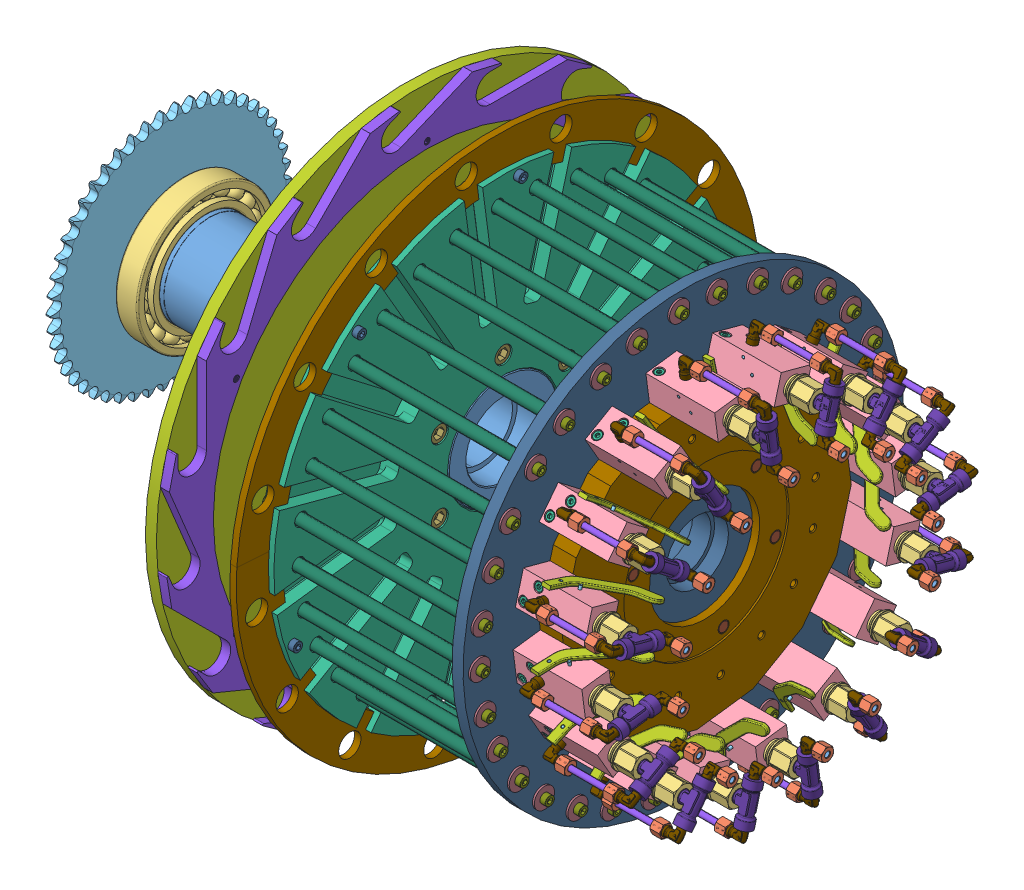
SolidWorks assembly assieme parte rotante, configuration Default. Lengths in mm.
Overall size (749.63 778.63 778.63).
555 component instances, 28 part files, 76 mates.
Components (placement in the parent):
- albero rotazione piatti-1: albero rotazione piatti [Default] at (60.413 18.3637 415) size (415 200 200)
- seger 100mm-2: seger 100mm [KS 1336 E - 100] at (-146.4567 18.3637 415) x (0 0 -1) z (1 0 0) size (107.55 112.98 3)
- SKF - 6020 - 20,DE,NC,20_68-1: SKF - 6020 - 20,DE,NC,20_68 [SKF - 6020 - 20,DE,NC,20_68] at (-131.4567 18.3637 415) x (1 0 0) z (0 -0.434476 -0.900684) size (24 150 150)
- calettatore d95-1: calettatore d95 [Default] at (-173.8867 18.3637 415) size (39.5 135 135)
- Chain wheel ISO - 50Z 10A-1-1: Chain wheel ISO - 50Z 10A-1 [Chain wheel ISO - 50Z 10A-1 --50SB120H25L95.0N] at (-164.8867 18.3637 415) size (28.93 262.06 262.51)
- Disco supporto montaggio e Colonne-1: Disco supporto montaggio e Colonne [Default] at (204.0433 18.3637 415) x (0 -0.866025 -0.5) z (1 0 0) size (499.6 499.6 29)
- SKF - 6020 - 20,DE,NC,20_68-2: SKF - 6020 - 20,DE,NC,20_68 [SKF - 6020 - 20,DE,NC,20_68] at (62.0433 18.3637 415) x (1 0 0) z (0 -0.432628 -0.901573) size (24 150 150)
- piatto rotante porta tappi-1: piatto rotante porta tappi [Default] at (99.0433 18.3637 415) x (0 0 -1) z (1 0 0) size (570 570 20.57)
- disco trasportatore tappi 31-1: disco trasportatore tappi 31 [Default] at (111.0433 18.3637 415) x (0 0.5 -0.866025) z (1 0 0) size (570 570 10.42)
- Distributore Rotante-1: Distributore Rotante [Default] at (425.0433 18.3637 415) x (0 -0.258819 -0.965926) z (1 0 0) size (310 310 25.54)
- disco trascinato porta distributore vuoto-1: disco trascinato porta distributore vuoto [Default] at (400.0433 18.3637 415) x (0 0.258819 0.965926) z (-1 0 0) size (480 480 50)
- m12 35mm-1: m12 35mm [ISO 4762 M12 x 35 - 35N] at (376.0433 -58.9104 394.2945) x (1 0 0) z (0 -0.5 0.866025) size (47 18 18)
- m12 90mm-3: m12 90mm [ISO 4762 M12 x 90 - 90N] at (203.0433 -21.6363 345.718) x (-1 0 0) z (0 -0.5 0.866025) size (102 18 18)
- rondella M6-90: rondella M6 [Washer ISO 7094 - 6] at (99.0433 -101.6363 207.1539) x (1 0 0) z (0 -1 0) size (2 22 22)
- M6 20mm-1: M6 20mm [ISO 4762 M6 x 20 - 20N] at (91.0433 -101.6363 207.1539) x (1 0 0) z (0 0.5 0.866025) size (26 10 10)
- m12 35mm-2: m12 35mm [ISO 4762 M12 x 35 - 35N] at (376.0433 -2.3418 337.7259) x (1 0 0) z (0 -1 0) size (47 18 18)
- m12 35mm-3: m12 35mm [ISO 4762 M12 x 35 - 35N] at (376.0433 74.9322 358.4315) x (1 0 0) z (0 -0.5 -0.866025) size (47 18 18)
- m12 35mm-4: m12 35mm [ISO 4762 M12 x 35 - 35N] at (376.0433 95.6378 435.7055) x (1 0 0) z (0 0.5 -0.866025) size (47 18 18)
- m12 35mm-5: m12 35mm [ISO 4762 M12 x 35 - 35N] at (376.0433 39.0692 492.2741) x (1 0 0) z (0 1 0) size (47 18 18)
- m12 35mm-6: m12 35mm [ISO 4762 M12 x 35 - 35N] at (376.0433 -38.2048 471.5685) x (1 0 0) z (0 0.5 0.866025) size (47 18 18)
- rondella M6-91: rondella M6 [Washer ISO 7094 - 6] at (99.0433 138.3637 207.1539) x (1 0 0) z (0 -0.5 -0.866025) size (2 22 22)
- rondella M6-92: rondella M6 [Washer ISO 7094 - 6] at (99.0433 258.3637 415) x (1 0 0) z (0 0.5 -0.866025) size (2 22 22)
- rondella M6-93: rondella M6 [Washer ISO 7094 - 6] at (99.0433 138.3637 622.8461) x (1 0 0) z (0 1 0) size (2 22 22)
- rondella M6-94: rondella M6 [Washer ISO 7094 - 6] at (99.0433 -101.6363 622.8461) x (1 0 0) z (0 0.5 0.866025) size (2 22 22)
- rondella M6-95: rondella M6 [Washer ISO 7094 - 6] at (99.0433 -221.6363 415) x (1 0 0) z (0 -0.5 0.866025) size (2 22 22)
- M6 20mm-2: M6 20mm [ISO 4762 M6 x 20 - 20N] at (91.0433 138.3637 207.1539) x (1 0 0) z (0 -0.5 0.866025) size (26 10 10)
- M6 20mm-3: M6 20mm [ISO 4762 M6 x 20 - 20N] at (91.0433 258.3637 415) x (1 0 0) z (0 -1 0) size (26 10 10)
- M6 20mm-4: M6 20mm [ISO 4762 M6 x 20 - 20N] at (91.0433 138.3637 622.8461) x (1 0 0) z (0 -0.5 -0.866025) size (26 10 10)
- M6 20mm-5: M6 20mm [ISO 4762 M6 x 20 - 20N] at (91.0433 -101.6363 622.8461) x (1 0 0) z (0 0.5 -0.866025) size (26 10 10)
- M6 20mm-6: M6 20mm [ISO 4762 M6 x 20 - 20N] at (91.0433 -221.6363 415) x (1 0 0) z (0 1 0) size (26 10 10)
- m12 90mm-4: m12 90mm [ISO 4762 M12 x 90 - 90N] at (203.0433 58.3637 345.718) x (-1 0 0) z (0 -1 0) size (102 18 18)
- m12 90mm-5: m12 90mm [ISO 4762 M12 x 90 - 90N] at (203.0433 98.3637 415) x (-1 0 0) z (0 -0.5 -0.866025) size (102 18 18)
- m12 90mm-6: m12 90mm [ISO 4762 M12 x 90 - 90N] at (203.0433 58.3637 484.282) x (-1 0 0) z (0 0.5 -0.866025) size (102 18 18)
- m12 90mm-7: m12 90mm [ISO 4762 M12 x 90 - 90N] at (203.0433 -21.6363 484.282) x (-1 0 0) z (0 1 0) size (102 18 18)
- m12 90mm-8: m12 90mm [ISO 4762 M12 x 90 - 90N] at (203.0433 -61.6363 415) x (-1 0 0) z (0 0.5 0.866025) size (102 18 18)
- asta scorrimento carello-1: asta scorrimento carello [Default] at (287.5433 70.1437 197.9013) x (0 0 -1) z (1 0 0) size (12 12 225)
- rondella M6-74: rondella M6 [Washer ISO 7094 - 6] at (175.0433 70.1437 197.9013) x (1 0 0) z (0 -1 0) size (2 22 22)
- M6 16mm-1: M6 16mm [ISO 4762 M6 x 16 - 16N] at (167.0433 70.1437 197.9013) size (22 10 10)
- M6 16mm-2: M6 16mm [ISO 4762 M6 x 16 - 16N] at (408.0433 70.1437 197.9013) x (-1 0 0) z (0 0 -1) size (22 10 10)
- rondella M6-96: rondella M6 [Washer ISO 7094 - 6] at (400.0433 70.1437 197.9013) x (-1 0 0) z (0 1 0) size (2 22 22)
- rondella M6-112: rondella M6 [Washer ISO 7094 - 6] at (175.0433 24.5373 191.8971) x (1 0 0) z (0 -0.965926 -0.258819) size (2 22 22)
- M6 16mm-3: M6 16mm [ISO 4762 M6 x 16 - 16N] at (167.0433 24.5373 191.8971) x (1 0 0) z (0 0.258819 -0.965926) size (22 10 10)
- asta scorrimento carello-2: asta scorrimento carello [Default] at (287.5433 24.5373 191.8971) x (0 0.258819 -0.965926) z (-1 0 0) size (12 12 225)
- rondella M6-128: rondella M6 [Washer ISO 7094 - 6] at (400.0433 24.5373 191.8971) x (-1 0 0) z (0 0.965926 0.258819) size (2 22 22)
- M6 16mm-4: M6 16mm [ISO 4762 M6 x 16 - 16N] at (408.0433 24.5373 191.8971) x (-1 0 0) z (0 -0.258819 0.965926) size (22 10 10)
- AssiemeValvola-1: AssiemeValvola [Default] at (515.3257 40.5532 246.4544) x (0 -0.130526 0.991445) z (0 0.991445 0.130526) size (90.26 138.63 38)
  - RaccordoT-1: RaccordoT [Default] at origin size (43 29.75 16.5)
  - Raccordo a L-1: Raccordo a L [Default] at (-30 0 0) x (0 -1 0) z (0 0 -1) size (28.34 25.51 14.01)
    - 1809_06_10_01-1: 1809_06_10_01 [Default] at origin size (22.49 23 10)
    - 1809_06_10_02-1: 1809_06_10_02 [Default] at origin size (6.5 8.5 8.5)
    - 1809_06_10_03-1: 1809_06_10_03 [Default] at origin size (11.02 15.01 14.01)
  - Raccordo a L-2: Raccordo a L [Default] at (30 0 0) x (0 1 0) z (0 0 -1) size (28.34 25.51 14.01)
    - 1809_06_10_01-1: 1809_06_10_01 [Default] at origin size (22.49 23 10)
    - 1809_06_10_02-1: 1809_06_10_02 [Default] at origin size (6.5 8.5 8.5)
    - 1809_06_10_03-1: 1809_06_10_03 [Default] at origin size (11.02 15.01 14.01)
  - TappoChiusura-1: TappoChiusura [Default] at (0 -32 0) x (0 -1 0) z (0 0 1) size (38.28 26.74 26.74)
  - CorpoValvola-1: CorpoValvola [Default] at (-15 -115.2824 0) size (30 75 34)
  - Raccordo a L-3: Raccordo a L [Default] at (-30 -88.2824 0) x (0 1 0) z (0 0 1) size (28.34 25.51 14.01)
    - 1809_06_10_01-1: 1809_06_10_01 [Default] at origin size (22.49 23 10)
    - 1809_06_10_02-1: 1809_06_10_02 [Default] at origin size (6.5 8.5 8.5)
    - 1809_06_10_03-1: 1809_06_10_03 [Default] at origin size (11.02 15.01 14.01)
  - Spina_3x38-1: Spina_3x38 [Default] at (0 -68.2824 -21) x (-1 0 0) z (0 0 1) size (3 3 38)
  - Spina_3x38-2: Spina_3x38 [Default] at (-10 -80.2824 -21) x (0.996193 0.087174 0) z (0 0 1) size (3 3 38)
  - M5 40mm-3: M5 40mm [ISO 4762 M5 x 40 - 40N] at (-14.6 -108.7824 9) size (45 8.5 8.5)
  - M5 40mm-2: M5 40mm [ISO 4762 M5 x 40 - 40N] at (-14.6 -96.7824 -9) size (45 8.5 8.5)
  - LevaValvola-1: LevaValvola [Default] at (-24.507 -86.571 -17) x (0.996193 0.087174 0) z (0 0 1) size (77.55 60.2 4)
  - Tubo-1: Tubo [Default] at (-30 -15.9665 0) x (1 0 0) z (0 -1 0) size (6 6 56.4)
- M6 16mm-5: M6 16mm [ISO 4762 M6 x 16 - 16N] at (167.0433 -16.8778 194.6116) x (1 0 0) z (0 0.382683 0.92388) size (22 10 10)
- M6 16mm-6: M6 16mm [ISO 4762 M6 x 16 - 16N] at (167.0433 -98.5342 224.874) x (1 0 0) z (0 0.707107 0.707107) size (22 10 10)
- M6 16mm-7: M6 16mm [ISO 4762 M6 x 16 - 16N] at (167.0433 -162.3939 284.0814) x (1 0 0) z (0 0.92388 0.382683) size (22 10 10)
- M6 16mm-8: M6 16mm [ISO 4762 M6 x 16 - 16N] at (167.0433 -198.735 363.22) x (1 0 0) z (0 1 0) size (22 10 10)
- M6 16mm-9: M6 16mm [ISO 4762 M6 x 16 - 16N] at (167.0433 -202.0247 450.2415) x (1 0 0) z (0 0.92388 -0.382683) size (22 10 10)
- M6 16mm-10: M6 16mm [ISO 4762 M6 x 16 - 16N] at (167.0433 -171.7623 531.8979) x (1 0 0) z (0 0.707107 -0.707107) size (22 10 10)
- M6 16mm-11: M6 16mm [ISO 4762 M6 x 16 - 16N] at (167.0433 -112.5549 595.7576) x (1 0 0) z (0 0.382683 -0.92388) size (22 10 10)
- M6 16mm-12: M6 16mm [ISO 4762 M6 x 16 - 16N] at (167.0433 -33.4163 632.0987) x (1 0 0) z (0 0 -1) size (22 10 10)
- M6 16mm-13: M6 16mm [ISO 4762 M6 x 16 - 16N] at (167.0433 53.6052 635.3884) x (1 0 0) z (0 -0.382683 -0.92388) size (22 10 10)
- M6 16mm-14: M6 16mm [ISO 4762 M6 x 16 - 16N] at (167.0433 135.2616 605.126) x (1 0 0) z (0 -0.707107 -0.707107) size (22 10 10)
- M6 16mm-15: M6 16mm [ISO 4762 M6 x 16 - 16N] at (167.0433 199.1213 545.9186) x (1 0 0) z (0 -0.92388 -0.382683) size (22 10 10)
- M6 16mm-16: M6 16mm [ISO 4762 M6 x 16 - 16N] at (167.0433 235.4624 466.78) x (1 0 0) z (0 -1 0) size (22 10 10)
- M6 16mm-17: M6 16mm [ISO 4762 M6 x 16 - 16N] at (167.0433 238.7521 379.7585) x (1 0 0) z (0 -0.92388 0.382683) size (22 10 10)
- M6 16mm-18: M6 16mm [ISO 4762 M6 x 16 - 16N] at (167.0433 208.4897 298.1021) x (1 0 0) z (0 -0.707107 0.707107) size (22 10 10)
- M6 16mm-19: M6 16mm [ISO 4762 M6 x 16 - 16N] at (167.0433 149.2823 234.2424) x (1 0 0) z (0 -0.382683 0.92388) size (22 10 10)
- rondella M6-75: rondella M6 [Washer ISO 7094 - 6] at (175.0433 -16.8778 194.6116) x (1 0 0) z (0 -0.92388 0.382683) size (2 22 22)
- rondella M6-76: rondella M6 [Washer ISO 7094 - 6] at (175.0433 -98.5342 224.874) x (1 0 0) z (0 -0.707107 0.707107) size (2 22 22)
- rondella M6-77: rondella M6 [Washer ISO 7094 - 6] at (175.0433 -162.3939 284.0814) x (1 0 0) z (0 -0.382683 0.92388) size (2 22 22)
- rondella M6-78: rondella M6 [Washer ISO 7094 - 6] at (175.0433 -198.735 363.22) size (2 22 22)
- rondella M6-79: rondella M6 [Washer ISO 7094 - 6] at (175.0433 -202.0247 450.2415) x (1 0 0) z (0 0.382683 0.92388) size (2 22 22)
- rondella M6-80: rondella M6 [Washer ISO 7094 - 6] at (175.0433 -171.7623 531.8979) x (1 0 0) z (0 0.707107 0.707107) size (2 22 22)
- rondella M6-81: rondella M6 [Washer ISO 7094 - 6] at (175.0433 -112.5549 595.7576) x (1 0 0) z (0 0.92388 0.382683) size (2 22 22)
- rondella M6-82: rondella M6 [Washer ISO 7094 - 6] at (175.0433 -33.4163 632.0987) x (1 0 0) z (0 1 0) size (2 22 22)
- rondella M6-83: rondella M6 [Washer ISO 7094 - 6] at (175.0433 53.6052 635.3884) x (1 0 0) z (0 0.92388 -0.382683) size (2 22 22)
- rondella M6-84: rondella M6 [Washer ISO 7094 - 6] at (175.0433 135.2616 605.126) x (1 0 0) z (0 0.707107 -0.707107) size (2 22 22)
- rondella M6-85: rondella M6 [Washer ISO 7094 - 6] at (175.0433 199.1213 545.9186) x (1 0 0) z (0 0.382683 -0.92388) size (2 22 22)
- rondella M6-86: rondella M6 [Washer ISO 7094 - 6] at (175.0433 235.4624 466.78) x (1 0 0) z (0 0 -1) size (2 22 22)
- rondella M6-87: rondella M6 [Washer ISO 7094 - 6] at (175.0433 238.7521 379.7585) x (1 0 0) z (0 -0.382683 -0.92388) size (2 22 22)
- rondella M6-88: rondella M6 [Washer ISO 7094 - 6] at (175.0433 208.4897 298.1021) x (1 0 0) z (0 -0.707107 -0.707107) size (2 22 22)
- rondella M6-89: rondella M6 [Washer ISO 7094 - 6] at (175.0433 149.2823 234.2424) x (1 0 0) z (0 -0.92388 -0.382683) size (2 22 22)
- asta scorrimento carello-3: asta scorrimento carello [Default] at (287.5433 -16.8778 194.6116) x (0 -0.382683 -0.92388) z (1 0 0) size (12 12 225)
- asta scorrimento carello-4: asta scorrimento carello [Default] at (287.5433 -98.5342 224.874) x (0 -0.707107 -0.707107) z (1 0 0) size (12 12 225)
- asta scorrimento carello-5: asta scorrimento carello [Default] at (287.5433 -162.3939 284.0814) x (0 -0.92388 -0.382683) z (1 0 0) size (12 12 225)
- asta scorrimento carello-6: asta scorrimento carello [Default] at (287.5433 -198.735 363.22) x (0 -1 0) z (1 0 0) size (12 12 225)
- asta scorrimento carello-7: asta scorrimento carello [Default] at (287.5433 -202.0247 450.2415) x (0 -0.92388 0.382683) z (1 0 0) size (12 12 225)
- asta scorrimento carello-8: asta scorrimento carello [Default] at (287.5433 -171.7623 531.8979) x (0 -0.707107 0.707107) z (1 0 0) size (12 12 225)
- asta scorrimento carello-9: asta scorrimento carello [Default] at (287.5433 -112.5549 595.7576) x (0 -0.382683 0.92388) z (1 0 0) size (12 12 225)
- asta scorrimento carello-10: asta scorrimento carello [Default] at (287.5433 -33.4163 632.0987) x (0 0 1) z (1 0 0) size (12 12 225)
- asta scorrimento carello-11: asta scorrimento carello [Default] at (287.5433 53.6052 635.3884) x (0 0.382683 0.92388) z (1 0 0) size (12 12 225)
- asta scorrimento carello-12: asta scorrimento carello [Default] at (287.5433 135.2616 605.126) x (0 0.707107 0.707107) z (1 0 0) size (12 12 225)
- asta scorrimento carello-13: asta scorrimento carello [Default] at (287.5433 199.1213 545.9186) x (0 0.92388 0.382683) z (1 0 0) size (12 12 225)
- asta scorrimento carello-14: asta scorrimento carello [Default] at (287.5433 235.4624 466.78) x (0 1 0) z (1 0 0) size (12 12 225)
- asta scorrimento carello-15: asta scorrimento carello [Default] at (287.5433 238.7521 379.7585) x (0 0.92388 -0.382683) z (1 0 0) size (12 12 225)
- asta scorrimento carello-16: asta scorrimento carello [Default] at (287.5433 208.4897 298.1021) x (0 0.707107 -0.707107) z (1 0 0) size (12 12 225)
- asta scorrimento carello-17: asta scorrimento carello [Default] at (287.5433 149.2823 234.2424) x (0 0.382683 -0.92388) z (1 0 0) size (12 12 225)
- M6 16mm-20: M6 16mm [ISO 4762 M6 x 16 - 16N] at (408.0433 -16.8778 194.6116) x (-1 0 0) z (0 -0.382683 -0.92388) size (22 10 10)
- M6 16mm-21: M6 16mm [ISO 4762 M6 x 16 - 16N] at (408.0433 -98.5342 224.874) x (-1 0 0) z (0 -0.707107 -0.707107) size (22 10 10)
- M6 16mm-22: M6 16mm [ISO 4762 M6 x 16 - 16N] at (408.0433 -162.3939 284.0814) x (-1 0 0) z (0 -0.92388 -0.382683) size (22 10 10)
- M6 16mm-23: M6 16mm [ISO 4762 M6 x 16 - 16N] at (408.0433 -198.735 363.22) x (-1 0 0) z (0 -1 0) size (22 10 10)
- M6 16mm-24: M6 16mm [ISO 4762 M6 x 16 - 16N] at (408.0433 -202.0247 450.2415) x (-1 0 0) z (0 -0.92388 0.382683) size (22 10 10)
- M6 16mm-25: M6 16mm [ISO 4762 M6 x 16 - 16N] at (408.0433 -171.7623 531.8979) x (-1 0 0) z (0 -0.707107 0.707107) size (22 10 10)
- M6 16mm-26: M6 16mm [ISO 4762 M6 x 16 - 16N] at (408.0433 -112.5549 595.7576) x (-1 0 0) z (0 -0.382683 0.92388) size (22 10 10)
- M6 16mm-27: M6 16mm [ISO 4762 M6 x 16 - 16N] at (408.0433 -33.4163 632.0987) x (-1 0 0) z (0 0 1) size (22 10 10)
- M6 16mm-28: M6 16mm [ISO 4762 M6 x 16 - 16N] at (408.0433 53.6052 635.3884) x (-1 0 0) z (0 0.382683 0.92388) size (22 10 10)
- M6 16mm-29: M6 16mm [ISO 4762 M6 x 16 - 16N] at (408.0433 135.2616 605.126) x (-1 0 0) z (0 0.707107 0.707107) size (22 10 10)
- M6 16mm-30: M6 16mm [ISO 4762 M6 x 16 - 16N] at (408.0433 199.1213 545.9186) x (-1 0 0) z (0 0.92388 0.382683) size (22 10 10)
- M6 16mm-31: M6 16mm [ISO 4762 M6 x 16 - 16N] at (408.0433 235.4624 466.78) x (-1 0 0) z (0 1 0) size (22 10 10)
- M6 16mm-32: M6 16mm [ISO 4762 M6 x 16 - 16N] at (408.0433 238.7521 379.7585) x (-1 0 0) z (0 0.92388 -0.382683) size (22 10 10)
- M6 16mm-33: M6 16mm [ISO 4762 M6 x 16 - 16N] at (408.0433 208.4897 298.1021) x (-1 0 0) z (0 0.707107 -0.707107) size (22 10 10)
- M6 16mm-34: M6 16mm [ISO 4762 M6 x 16 - 16N] at (408.0433 149.2823 234.2424) x (-1 0 0) z (0 0.382683 -0.92388) size (22 10 10)
- rondella M6-97: rondella M6 [Washer ISO 7094 - 6] at (400.0433 -16.8778 194.6116) x (-1 0 0) z (0 0.92388 -0.382683) size (2 22 22)
- rondella M6-98: rondella M6 [Washer ISO 7094 - 6] at (400.0433 -98.5342 224.874) x (-1 0 0) z (0 0.707107 -0.707107) size (2 22 22)
- rondella M6-99: rondella M6 [Washer ISO 7094 - 6] at (400.0433 -162.3939 284.0814) x (-1 0 0) z (0 0.382683 -0.92388) size (2 22 22)
- rondella M6-100: rondella M6 [Washer ISO 7094 - 6] at (400.0433 -198.735 363.22) x (-1 0 0) z (0 0 -1) size (2 22 22)
- rondella M6-101: rondella M6 [Washer ISO 7094 - 6] at (400.0433 -202.0247 450.2415) x (-1 0 0) z (0 -0.382683 -0.92388) size (2 22 22)
- rondella M6-102: rondella M6 [Washer ISO 7094 - 6] at (400.0433 -171.7623 531.8979) x (-1 0 0) z (0 -0.707107 -0.707107) size (2 22 22)
- rondella M6-103: rondella M6 [Washer ISO 7094 - 6] at (400.0433 -112.5549 595.7576) x (-1 0 0) z (0 -0.92388 -0.382683) size (2 22 22)
- rondella M6-104: rondella M6 [Washer ISO 7094 - 6] at (400.0433 -33.4163 632.0987) x (-1 0 0) z (0 -1 0) size (2 22 22)
- rondella M6-105: rondella M6 [Washer ISO 7094 - 6] at (400.0433 53.6052 635.3884) x (-1 0 0) z (0 -0.92388 0.382683) size (2 22 22)
- rondella M6-106: rondella M6 [Washer ISO 7094 - 6] at (400.0433 135.2616 605.126) x (-1 0 0) z (0 -0.707107 0.707107) size (2 22 22)
- rondella M6-107: rondella M6 [Washer ISO 7094 - 6] at (400.0433 199.1213 545.9186) x (-1 0 0) z (0 -0.382683 0.92388) size (2 22 22)
- rondella M6-108: rondella M6 [Washer ISO 7094 - 6] at (400.0433 235.4624 466.78) x (-1 0 0) z (0 0 1) size (2 22 22)
- rondella M6-109: rondella M6 [Washer ISO 7094 - 6] at (400.0433 238.7521 379.7585) x (-1 0 0) z (0 0.382683 0.92388) size (2 22 22)
- rondella M6-110: rondella M6 [Washer ISO 7094 - 6] at (400.0433 208.4897 298.1021) x (-1 0 0) z (0 0.707107 0.707107) size (2 22 22)
- rondella M6-111: rondella M6 [Washer ISO 7094 - 6] at (400.0433 149.2823 234.2424) x (-1 0 0) z (0 0.92388 0.382683) size (2 22 22)
- rondella M6-113: rondella M6 [Washer ISO 7094 - 6] at (175.0433 -61.3104 206.5173) x (1 0 0) z (0 -0.991445 0.130526) size (2 22 22)
- rondella M6-114: rondella M6 [Washer ISO 7094 - 6] at (175.0433 -135.0285 252.8771) x (1 0 0) z (0 -0.866025 0.5) size (2 22 22)
- rondella M6-115: rondella M6 [Washer ISO 7094 - 6] at (175.0433 -185.3939 323.9186) x (1 0 0) z (0 -0.608761 0.793353) size (2 22 22)
- rondella M6-116: rondella M6 [Washer ISO 7094 - 6] at (175.0433 -204.7392 408.8264) x (1 0 0) z (0 -0.258819 0.965926) size (2 22 22)
- rondella M6-117: rondella M6 [Washer ISO 7094 - 6] at (175.0433 -190.119 494.6741) x (1 0 0) z (0 0.130526 0.991445) size (2 22 22)
- rondella M6-118: rondella M6 [Washer ISO 7094 - 6] at (175.0433 -143.7592 568.3922) x (1 0 0) z (0 0.5 0.866025) size (2 22 22)
- rondella M6-119: rondella M6 [Washer ISO 7094 - 6] at (175.0433 -72.7177 618.7576) x (1 0 0) z (0 0.793353 0.608761) size (2 22 22)
- rondella M6-120: rondella M6 [Washer ISO 7094 - 6] at (175.0433 12.1901 638.1029) x (1 0 0) z (0 0.965926 0.258819) size (2 22 22)
- rondella M6-121: rondella M6 [Washer ISO 7094 - 6] at (175.0433 98.0378 623.4827) x (1 0 0) z (0 0.991445 -0.130526) size (2 22 22)
- rondella M6-122: rondella M6 [Washer ISO 7094 - 6] at (175.0433 171.7559 577.1229) x (1 0 0) z (0 0.866025 -0.5) size (2 22 22)
- rondella M6-123: rondella M6 [Washer ISO 7094 - 6] at (175.0433 222.1213 506.0814) x (1 0 0) z (0 0.608761 -0.793353) size (2 22 22)
- rondella M6-124: rondella M6 [Washer ISO 7094 - 6] at (175.0433 241.4666 421.1736) x (1 0 0) z (0 0.258819 -0.965926) size (2 22 22)
- rondella M6-125: rondella M6 [Washer ISO 7094 - 6] at (175.0433 226.8464 335.3259) x (1 0 0) z (0 -0.130526 -0.991445) size (2 22 22)
- rondella M6-126: rondella M6 [Washer ISO 7094 - 6] at (175.0433 180.4866 261.6078) x (1 0 0) z (0 -0.5 -0.866025) size (2 22 22)
- rondella M6-127: rondella M6 [Washer ISO 7094 - 6] at (175.0433 109.4451 211.2424) x (1 0 0) z (0 -0.793353 -0.608761) size (2 22 22)
- M6 16mm-35: M6 16mm [ISO 4762 M6 x 16 - 16N] at (167.0433 -61.3104 206.5173) x (1 0 0) z (0 -0.130526 -0.991445) size (22 10 10)
- M6 16mm-36: M6 16mm [ISO 4762 M6 x 16 - 16N] at (167.0433 -135.0285 252.8771) x (1 0 0) z (0 -0.5 -0.866025) size (22 10 10)
- M6 16mm-37: M6 16mm [ISO 4762 M6 x 16 - 16N] at (167.0433 -185.3939 323.9186) x (1 0 0) z (0 -0.793353 -0.608761) size (22 10 10)
- M6 16mm-38: M6 16mm [ISO 4762 M6 x 16 - 16N] at (167.0433 -204.7392 408.8264) x (1 0 0) z (0 -0.965926 -0.258819) size (22 10 10)
- M6 16mm-39: M6 16mm [ISO 4762 M6 x 16 - 16N] at (167.0433 -190.119 494.6741) x (1 0 0) z (0 -0.991445 0.130526) size (22 10 10)
- M6 16mm-40: M6 16mm [ISO 4762 M6 x 16 - 16N] at (167.0433 -143.7592 568.3922) x (1 0 0) z (0 -0.866025 0.5) size (22 10 10)
- M6 16mm-41: M6 16mm [ISO 4762 M6 x 16 - 16N] at (167.0433 -72.7177 618.7576) x (1 0 0) z (0 -0.608761 0.793353) size (22 10 10)
- M6 16mm-42: M6 16mm [ISO 4762 M6 x 16 - 16N] at (167.0433 12.1901 638.1029) x (1 0 0) z (0 -0.258819 0.965926) size (22 10 10)
- M6 16mm-43: M6 16mm [ISO 4762 M6 x 16 - 16N] at (167.0433 98.0378 623.4827) x (1 0 0) z (0 0.130526 0.991445) size (22 10 10)
- M6 16mm-44: M6 16mm [ISO 4762 M6 x 16 - 16N] at (167.0433 171.7559 577.1229) x (1 0 0) z (0 0.5 0.866025) size (22 10 10)
- M6 16mm-45: M6 16mm [ISO 4762 M6 x 16 - 16N] at (167.0433 222.1213 506.0814) x (1 0 0) z (0 0.793353 0.608761) size (22 10 10)
- M6 16mm-46: M6 16mm [ISO 4762 M6 x 16 - 16N] at (167.0433 241.4666 421.1736) x (1 0 0) z (0 0.965926 0.258819) size (22 10 10)
- M6 16mm-47: M6 16mm [ISO 4762 M6 x 16 - 16N] at (167.0433 226.8464 335.3259) x (1 0 0) z (0 0.991445 -0.130526) size (22 10 10)
- M6 16mm-48: M6 16mm [ISO 4762 M6 x 16 - 16N] at (167.0433 180.4866 261.6078) x (1 0 0) z (0 0.866025 -0.5) size (22 10 10)
- M6 16mm-49: M6 16mm [ISO 4762 M6 x 16 - 16N] at (167.0433 109.4451 211.2424) x (1 0 0) z (0 0.608761 -0.793353) size (22 10 10)
- asta scorrimento carello-18: asta scorrimento carello [Default] at (287.5433 -61.3104 206.5173) x (0 -0.130526 -0.991445) z (-1 0 0) size (12 12 225)
- asta scorrimento carello-19: asta scorrimento carello [Default] at (287.5433 -135.0285 252.8771) x (0 -0.5 -0.866025) z (-1 0 0) size (12 12 225)
- asta scorrimento carello-20: asta scorrimento carello [Default] at (287.5433 -185.3939 323.9186) x (0 -0.793353 -0.608761) z (-1 0 0) size (12 12 225)
- asta scorrimento carello-21: asta scorrimento carello [Default] at (287.5433 -204.7392 408.8264) x (0 -0.965926 -0.258819) z (-1 0 0) size (12 12 225)
- asta scorrimento carello-22: asta scorrimento carello [Default] at (287.5433 -190.119 494.6741) x (0 -0.991445 0.130526) z (-1 0 0) size (12 12 225)
- asta scorrimento carello-23: asta scorrimento carello [Default] at (287.5433 -143.7592 568.3922) x (0 -0.866025 0.5) z (-1 0 0) size (12 12 225)
- asta scorrimento carello-24: asta scorrimento carello [Default] at (287.5433 -72.7177 618.7576) x (0 -0.608761 0.793353) z (-1 0 0) size (12 12 225)
- asta scorrimento carello-25: asta scorrimento carello [Default] at (287.5433 12.1901 638.1029) x (0 -0.258819 0.965926) z (-1 0 0) size (12 12 225)
- asta scorrimento carello-26: asta scorrimento carello [Default] at (287.5433 98.0378 623.4827) x (0 0.130526 0.991445) z (-1 0 0) size (12 12 225)
- asta scorrimento carello-27: asta scorrimento carello [Default] at (287.5433 171.7559 577.1229) x (0 0.5 0.866025) z (-1 0 0) size (12 12 225)
- asta scorrimento carello-28: asta scorrimento carello [Default] at (287.5433 222.1213 506.0814) x (0 0.793353 0.608761) z (-1 0 0) size (12 12 225)
- asta scorrimento carello-29: asta scorrimento carello [Default] at (287.5433 241.4666 421.1736) x (0 0.965926 0.258819) z (-1 0 0) size (12 12 225)
- asta scorrimento carello-30: asta scorrimento carello [Default] at (287.5433 226.8464 335.3259) x (0 0.991445 -0.130526) z (-1 0 0) size (12 12 225)
- asta scorrimento carello-31: asta scorrimento carello [Default] at (287.5433 180.4866 261.6078) x (0 0.866025 -0.5) z (-1 0 0) size (12 12 225)
- asta scorrimento carello-32: asta scorrimento carello [Default] at (287.5433 109.4451 211.2424) x (0 0.608761 -0.793353) z (-1 0 0) size (12 12 225)
- rondella M6-129: rondella M6 [Washer ISO 7094 - 6] at (400.0433 -61.3104 206.5173) x (-1 0 0) z (0 0.991445 -0.130526) size (2 22 22)
- rondella M6-130: rondella M6 [Washer ISO 7094 - 6] at (400.0433 -135.0285 252.8771) x (-1 0 0) z (0 0.866025 -0.5) size (2 22 22)
- rondella M6-131: rondella M6 [Washer ISO 7094 - 6] at (400.0433 -185.3939 323.9186) x (-1 0 0) z (0 0.608761 -0.793353) size (2 22 22)
- rondella M6-132: rondella M6 [Washer ISO 7094 - 6] at (400.0433 -204.7392 408.8264) x (-1 0 0) z (0 0.258819 -0.965926) size (2 22 22)
- rondella M6-133: rondella M6 [Washer ISO 7094 - 6] at (400.0433 -190.119 494.6741) x (-1 0 0) z (0 -0.130526 -0.991445) size (2 22 22)
- rondella M6-134: rondella M6 [Washer ISO 7094 - 6] at (400.0433 -143.7592 568.3922) x (-1 0 0) z (0 -0.5 -0.866025) size (2 22 22)
- rondella M6-135: rondella M6 [Washer ISO 7094 - 6] at (400.0433 -72.7177 618.7576) x (-1 0 0) z (0 -0.793353 -0.608761) size (2 22 22)
- rondella M6-136: rondella M6 [Washer ISO 7094 - 6] at (400.0433 12.1901 638.1029) x (-1 0 0) z (0 -0.965926 -0.258819) size (2 22 22)
- rondella M6-137: rondella M6 [Washer ISO 7094 - 6] at (400.0433 98.0378 623.4827) x (-1 0 0) z (0 -0.991445 0.130526) size (2 22 22)
- rondella M6-138: rondella M6 [Washer ISO 7094 - 6] at (400.0433 171.7559 577.1229) x (-1 0 0) z (0 -0.866025 0.5) size (2 22 22)
- rondella M6-139: rondella M6 [Washer ISO 7094 - 6] at (400.0433 222.1213 506.0814) x (-1 0 0) z (0 -0.608761 0.793353) size (2 22 22)
- rondella M6-140: rondella M6 [Washer ISO 7094 - 6] at (400.0433 241.4666 421.1736) x (-1 0 0) z (0 -0.258819 0.965926) size (2 22 22)
- rondella M6-141: rondella M6 [Washer ISO 7094 - 6] at (400.0433 226.8464 335.3259) x (-1 0 0) z (0 0.130526 0.991445) size (2 22 22)
- rondella M6-142: rondella M6 [Washer ISO 7094 - 6] at (400.0433 180.4866 261.6078) x (-1 0 0) z (0 0.5 0.866025) size (2 22 22)
- rondella M6-143: rondella M6 [Washer ISO 7094 - 6] at (400.0433 109.4451 211.2424) x (-1 0 0) z (0 0.793353 0.608761) size (2 22 22)
- M6 16mm-50: M6 16mm [ISO 4762 M6 x 16 - 16N] at (408.0433 -61.3104 206.5173) x (-1 0 0) z (0 0.130526 0.991445) size (22 10 10)
- M6 16mm-51: M6 16mm [ISO 4762 M6 x 16 - 16N] at (408.0433 -135.0285 252.8771) x (-1 0 0) z (0 0.5 0.866025) size (22 10 10)
- M6 16mm-52: M6 16mm [ISO 4762 M6 x 16 - 16N] at (408.0433 -185.3939 323.9186) x (-1 0 0) z (0 0.793353 0.608761) size (22 10 10)
- M6 16mm-53: M6 16mm [ISO 4762 M6 x 16 - 16N] at (408.0433 -204.7392 408.8264) x (-1 0 0) z (0 0.965926 0.258819) size (22 10 10)
- M6 16mm-54: M6 16mm [ISO 4762 M6 x 16 - 16N] at (408.0433 -190.119 494.6741) x (-1 0 0) z (0 0.991445 -0.130526) size (22 10 10)
- M6 16mm-55: M6 16mm [ISO 4762 M6 x 16 - 16N] at (408.0433 -143.7592 568.3922) x (-1 0 0) z (0 0.866025 -0.5) size (22 10 10)
- M6 16mm-56: M6 16mm [ISO 4762 M6 x 16 - 16N] at (408.0433 -72.7177 618.7576) x (-1 0 0) z (0 0.608761 -0.793353) size (22 10 10)
- M6 16mm-57: M6 16mm [ISO 4762 M6 x 16 - 16N] at (408.0433 12.1901 638.1029) x (-1 0 0) z (0 0.258819 -0.965926) size (22 10 10)
- M6 16mm-58: M6 16mm [ISO 4762 M6 x 16 - 16N] at (408.0433 98.0378 623.4827) x (-1 0 0) z (0 -0.130526 -0.991445) size (22 10 10)
- M6 16mm-59: M6 16mm [ISO 4762 M6 x 16 - 16N] at (408.0433 171.7559 577.1229) x (-1 0 0) z (0 -0.5 -0.866025) size (22 10 10)
- M6 16mm-60: M6 16mm [ISO 4762 M6 x 16 - 16N] at (408.0433 222.1213 506.0814) x (-1 0 0) z (0 -0.793353 -0.608761) size (22 10 10)
- M6 16mm-61: M6 16mm [ISO 4762 M6 x 16 - 16N] at (408.0433 241.4666 421.1736) x (-1 0 0) z (0 -0.965926 -0.258819) size (22 10 10)
- M6 16mm-62: M6 16mm [ISO 4762 M6 x 16 - 16N] at (408.0433 226.8464 335.3259) x (-1 0 0) z (0 -0.991445 0.130526) size (22 10 10)
- M6 16mm-63: M6 16mm [ISO 4762 M6 x 16 - 16N] at (408.0433 180.4866 261.6078) x (-1 0 0) z (0 -0.866025 0.5) size (22 10 10)
- M6 16mm-64: M6 16mm [ISO 4762 M6 x 16 - 16N] at (408.0433 109.4451 211.2424) x (-1 0 0) z (0 -0.608761 0.793353) size (22 10 10)
- AssiemeValvola-2: AssiemeValvola [Default] at (515.3257 -25.6355 250.7926) x (0 0.258819 0.965926) z (0 0.965926 -0.258819) size (90.26 138.63 38)
  - RaccordoT-1: RaccordoT [Default] at origin size (43 29.75 16.5)
  - Raccordo a L-1: Raccordo a L [Default] at (-30 0 0) x (0 -1 0) z (0 0 -1) size (28.34 25.51 14.01)
    - 1809_06_10_01-1: 1809_06_10_01 [Default] at origin size (22.49 23 10)
    - 1809_06_10_02-1: 1809_06_10_02 [Default] at origin size (6.5 8.5 8.5)
    - 1809_06_10_03-1: 1809_06_10_03 [Default] at origin size (11.02 15.01 14.01)
  - Raccordo a L-2: Raccordo a L [Default] at (30 0 0) x (0 1 0) z (0 0 -1) size (28.34 25.51 14.01)
    - 1809_06_10_01-1: 1809_06_10_01 [Default] at origin size (22.49 23 10)
    - 1809_06_10_02-1: 1809_06_10_02 [Default] at origin size (6.5 8.5 8.5)
    - 1809_06_10_03-1: 1809_06_10_03 [Default] at origin size (11.02 15.01 14.01)
  - TappoChiusura-1: TappoChiusura [Default] at (0 -32 0) x (0 -1 0) z (0 0 1) size (38.28 26.74 26.74)
  - CorpoValvola-1: CorpoValvola [Default] at (-15 -115.2824 0) size (30 75 34)
  - Raccordo a L-3: Raccordo a L [Default] at (-30 -88.2824 0) x (0 1 0) z (0 0 1) size (28.34 25.51 14.01)
    - 1809_06_10_01-1: 1809_06_10_01 [Default] at origin size (22.49 23 10)
    - 1809_06_10_02-1: 1809_06_10_02 [Default] at origin size (6.5 8.5 8.5)
    - 1809_06_10_03-1: 1809_06_10_03 [Default] at origin size (11.02 15.01 14.01)
  - Spina_3x38-1: Spina_3x38 [Default] at (0 -68.2824 -21) x (-1 0 0) z (0 0 1) size (3 3 38)
  - Spina_3x38-2: Spina_3x38 [Default] at (-10 -80.2824 -21) x (0.996193 0.087174 0) z (0 0 1) size (3 3 38)
  - M5 40mm-3: M5 40mm [ISO 4762 M5 x 40 - 40N] at (-14.6 -108.7824 9) size (45 8.5 8.5)
  - M5 40mm-2: M5 40mm [ISO 4762 M5 x 40 - 40N] at (-14.6 -96.7824 -9) size (45 8.5 8.5)
  - LevaValvola-1: LevaValvola [Default] at (-24.507 -86.571 -17) x (0.996193 0.087174 0) z (0 0 1) size (77.55 60.2 4)
  - Tubo-1: Tubo [Default] at (-30 -15.9665 0) x (1 0 0) z (0 -1 0) size (6 6 56.4)
- AssiemeValvola-3: AssiemeValvola [Default] at (515.3257 -85.1257 280.1299) x (0 0.608761 0.793353) z (0 0.793353 -0.608761) size (90.26 138.63 38)
  - RaccordoT-1: RaccordoT [Default] at origin size (43 29.75 16.5)
  - Raccordo a L-1: Raccordo a L [Default] at (-30 0 0) x (0 -1 0) z (0 0 -1) size (28.34 25.51 14.01)
    - 1809_06_10_01-1: 1809_06_10_01 [Default] at origin size (22.49 23 10)
    - 1809_06_10_02-1: 1809_06_10_02 [Default] at origin size (6.5 8.5 8.5)
    - 1809_06_10_03-1: 1809_06_10_03 [Default] at origin size (11.02 15.01 14.01)
  - Raccordo a L-2: Raccordo a L [Default] at (30 0 0) x (0 1 0) z (0 0 -1) size (28.34 25.51 14.01)
    - 1809_06_10_01-1: 1809_06_10_01 [Default] at origin size (22.49 23 10)
    - 1809_06_10_02-1: 1809_06_10_02 [Default] at origin size (6.5 8.5 8.5)
    - 1809_06_10_03-1: 1809_06_10_03 [Default] at origin size (11.02 15.01 14.01)
  - TappoChiusura-1: TappoChiusura [Default] at (0 -32 0) x (0 -1 0) z (0 0 1) size (38.28 26.74 26.74)
  - CorpoValvola-1: CorpoValvola [Default] at (-15 -115.2824 0) size (30 75 34)
  - Raccordo a L-3: Raccordo a L [Default] at (-30 -88.2824 0) x (0 1 0) z (0 0 1) size (28.34 25.51 14.01)
    - 1809_06_10_01-1: 1809_06_10_01 [Default] at origin size (22.49 23 10)
    - 1809_06_10_02-1: 1809_06_10_02 [Default] at origin size (6.5 8.5 8.5)
    - 1809_06_10_03-1: 1809_06_10_03 [Default] at origin size (11.02 15.01 14.01)
  - Spina_3x38-1: Spina_3x38 [Default] at (0 -68.2824 -21) x (-1 0 0) z (0 0 1) size (3 3 38)
  - Spina_3x38-2: Spina_3x38 [Default] at (-10 -80.2824 -21) x (0.996193 0.087174 0) z (0 0 1) size (3 3 38)
  - M5 40mm-3: M5 40mm [ISO 4762 M5 x 40 - 40N] at (-14.6 -108.7824 9) size (45 8.5 8.5)
  - M5 40mm-2: M5 40mm [ISO 4762 M5 x 40 - 40N] at (-14.6 -96.7824 -9) size (45 8.5 8.5)
  - LevaValvola-1: LevaValvola [Default] at (-24.507 -86.571 -17) x (0.996193 0.087174 0) z (0 0 1) size (77.55 60.2 4)
  - Tubo-1: Tubo [Default] at (-30 -15.9665 0) x (1 0 0) z (0 -1 0) size (6 6 56.4)
- AssiemeValvola-4: AssiemeValvola [Default] at (515.3257 -128.8606 330) x (0 0.866025 0.5) z (0 0.5 -0.866025) size (90.26 138.63 38)
  - RaccordoT-1: RaccordoT [Default] at origin size (43 29.75 16.5)
  - Raccordo a L-1: Raccordo a L [Default] at (-30 0 0) x (0 -1 0) z (0 0 -1) size (28.34 25.51 14.01)
    - 1809_06_10_01-1: 1809_06_10_01 [Default] at origin size (22.49 23 10)
    - 1809_06_10_02-1: 1809_06_10_02 [Default] at origin size (6.5 8.5 8.5)
    - 1809_06_10_03-1: 1809_06_10_03 [Default] at origin size (11.02 15.01 14.01)
  - Raccordo a L-2: Raccordo a L [Default] at (30 0 0) x (0 1 0) z (0 0 -1) size (28.34 25.51 14.01)
    - 1809_06_10_01-1: 1809_06_10_01 [Default] at origin size (22.49 23 10)
    - 1809_06_10_02-1: 1809_06_10_02 [Default] at origin size (6.5 8.5 8.5)
    - 1809_06_10_03-1: 1809_06_10_03 [Default] at origin size (11.02 15.01 14.01)
  - TappoChiusura-1: TappoChiusura [Default] at (0 -32 0) x (0 -1 0) z (0 0 1) size (38.28 26.74 26.74)
  - CorpoValvola-1: CorpoValvola [Default] at (-15 -115.2824 0) size (30 75 34)
  - Raccordo a L-3: Raccordo a L [Default] at (-30 -88.2824 0) x (0 1 0) z (0 0 1) size (28.34 25.51 14.01)
    - 1809_06_10_01-1: 1809_06_10_01 [Default] at origin size (22.49 23 10)
    - 1809_06_10_02-1: 1809_06_10_02 [Default] at origin size (6.5 8.5 8.5)
    - 1809_06_10_03-1: 1809_06_10_03 [Default] at origin size (11.02 15.01 14.01)
  - Spina_3x38-1: Spina_3x38 [Default] at (0 -68.2824 -21) x (-1 0 0) z (0 0 1) size (3 3 38)
  - Spina_3x38-2: Spina_3x38 [Default] at (-10 -80.2824 -21) x (0.996193 0.087174 0) z (0 0 1) size (3 3 38)
  - M5 40mm-3: M5 40mm [ISO 4762 M5 x 40 - 40N] at (-14.6 -108.7824 9) size (45 8.5 8.5)
  - M5 40mm-2: M5 40mm [ISO 4762 M5 x 40 - 40N] at (-14.6 -96.7824 -9) size (45 8.5 8.5)
  - LevaValvola-1: LevaValvola [Default] at (-24.507 -86.571 -17) x (0.996193 0.087174 0) z (0 0 1) size (77.55 60.2 4)
  - Tubo-1: Tubo [Default] at (-30 -15.9665 0) x (1 0 0) z (0 -1 0) size (6 6 56.4)
- AssiemeValvola-5: AssiemeValvola [Default] at (515.3257 -150.1819 392.8105) x (0 0.991445 0.130526) z (0 0.130526 -0.991445) size (90.26 138.63 38)
  - RaccordoT-1: RaccordoT [Default] at origin size (43 29.75 16.5)
  - Raccordo a L-1: Raccordo a L [Default] at (-30 0 0) x (0 -1 0) z (0 0 -1) size (28.34 25.51 14.01)
    - 1809_06_10_01-1: 1809_06_10_01 [Default] at origin size (22.49 23 10)
    - 1809_06_10_02-1: 1809_06_10_02 [Default] at origin size (6.5 8.5 8.5)
    - 1809_06_10_03-1: 1809_06_10_03 [Default] at origin size (11.02 15.01 14.01)
  - Raccordo a L-2: Raccordo a L [Default] at (30 0 0) x (0 1 0) z (0 0 -1) size (28.34 25.51 14.01)
    - 1809_06_10_01-1: 1809_06_10_01 [Default] at origin size (22.49 23 10)
    - 1809_06_10_02-1: 1809_06_10_02 [Default] at origin size (6.5 8.5 8.5)
    - 1809_06_10_03-1: 1809_06_10_03 [Default] at origin size (11.02 15.01 14.01)
  - TappoChiusura-1: TappoChiusura [Default] at (0 -32 0) x (0 -1 0) z (0 0 1) size (38.28 26.74 26.74)
  - CorpoValvola-1: CorpoValvola [Default] at (-15 -115.2824 0) size (30 75 34)
  - Raccordo a L-3: Raccordo a L [Default] at (-30 -88.2824 0) x (0 1 0) z (0 0 1) size (28.34 25.51 14.01)
    - 1809_06_10_01-1: 1809_06_10_01 [Default] at origin size (22.49 23 10)
    - 1809_06_10_02-1: 1809_06_10_02 [Default] at origin size (6.5 8.5 8.5)
    - 1809_06_10_03-1: 1809_06_10_03 [Default] at origin size (11.02 15.01 14.01)
  - Spina_3x38-1: Spina_3x38 [Default] at (0 -68.2824 -21) x (-1 0 0) z (0 0 1) size (3 3 38)
  - Spina_3x38-2: Spina_3x38 [Default] at (-10 -80.2824 -21) x (0.996193 0.087174 0) z (0 0 1) size (3 3 38)
  - M5 40mm-3: M5 40mm [ISO 4762 M5 x 40 - 40N] at (-14.6 -108.7824 9) size (45 8.5 8.5)
  - M5 40mm-2: M5 40mm [ISO 4762 M5 x 40 - 40N] at (-14.6 -96.7824 -9) size (45 8.5 8.5)
  - LevaValvola-1: LevaValvola [Default] at (-24.507 -86.571 -17) x (0.996193 0.087174 0) z (0 0 1) size (77.55 60.2 4)
  - Tubo-1: Tubo [Default] at (-30 -15.9665 0) x (1 0 0) z (0 -1 0) size (6 6 56.4)
- AssiemeValvola-6: AssiemeValvola [Default] at (515.3257 -145.8437 458.9992) x (0 0.965926 -0.258819) z (0 -0.258819 -0.965926) size (90.26 138.63 38)
  - RaccordoT-1: RaccordoT [Default] at origin size (43 29.75 16.5)
  - Raccordo a L-1: Raccordo a L [Default] at (-30 0 0) x (0 -1 0) z (0 0 -1) size (28.34 25.51 14.01)
    - 1809_06_10_01-1: 1809_06_10_01 [Default] at origin size (22.49 23 10)
    - 1809_06_10_02-1: 1809_06_10_02 [Default] at origin size (6.5 8.5 8.5)
    - 1809_06_10_03-1: 1809_06_10_03 [Default] at origin size (11.02 15.01 14.01)
  - Raccordo a L-2: Raccordo a L [Default] at (30 0 0) x (0 1 0) z (0 0 -1) size (28.34 25.51 14.01)
    - 1809_06_10_01-1: 1809_06_10_01 [Default] at origin size (22.49 23 10)
    - 1809_06_10_02-1: 1809_06_10_02 [Default] at origin size (6.5 8.5 8.5)
    - 1809_06_10_03-1: 1809_06_10_03 [Default] at origin size (11.02 15.01 14.01)
  - TappoChiusura-1: TappoChiusura [Default] at (0 -32 0) x (0 -1 0) z (0 0 1) size (38.28 26.74 26.74)
  - CorpoValvola-1: CorpoValvola [Default] at (-15 -115.2824 0) size (30 75 34)
  - Raccordo a L-3: Raccordo a L [Default] at (-30 -88.2824 0) x (0 1 0) z (0 0 1) size (28.34 25.51 14.01)
    - 1809_06_10_01-1: 1809_06_10_01 [Default] at origin size (22.49 23 10)
    - 1809_06_10_02-1: 1809_06_10_02 [Default] at origin size (6.5 8.5 8.5)
    - 1809_06_10_03-1: 1809_06_10_03 [Default] at origin size (11.02 15.01 14.01)
  - Spina_3x38-1: Spina_3x38 [Default] at (0 -68.2824 -21) x (-1 0 0) z (0 0 1) size (3 3 38)
  - Spina_3x38-2: Spina_3x38 [Default] at (-10 -80.2824 -21) x (0.996193 0.087174 0) z (0 0 1) size (3 3 38)
  - M5 40mm-3: M5 40mm [ISO 4762 M5 x 40 - 40N] at (-14.6 -108.7824 9) size (45 8.5 8.5)
  - M5 40mm-2: M5 40mm [ISO 4762 M5 x 40 - 40N] at (-14.6 -96.7824 -9) size (45 8.5 8.5)
  - LevaValvola-1: LevaValvola [Default] at (-24.507 -86.571 -17) x (0.996193 0.087174 0) z (0 0 1) size (77.55 60.2 4)
  - Tubo-1: Tubo [Default] at (-30 -15.9665 0) x (1 0 0) z (0 -1 0) size (6 6 56.4)
